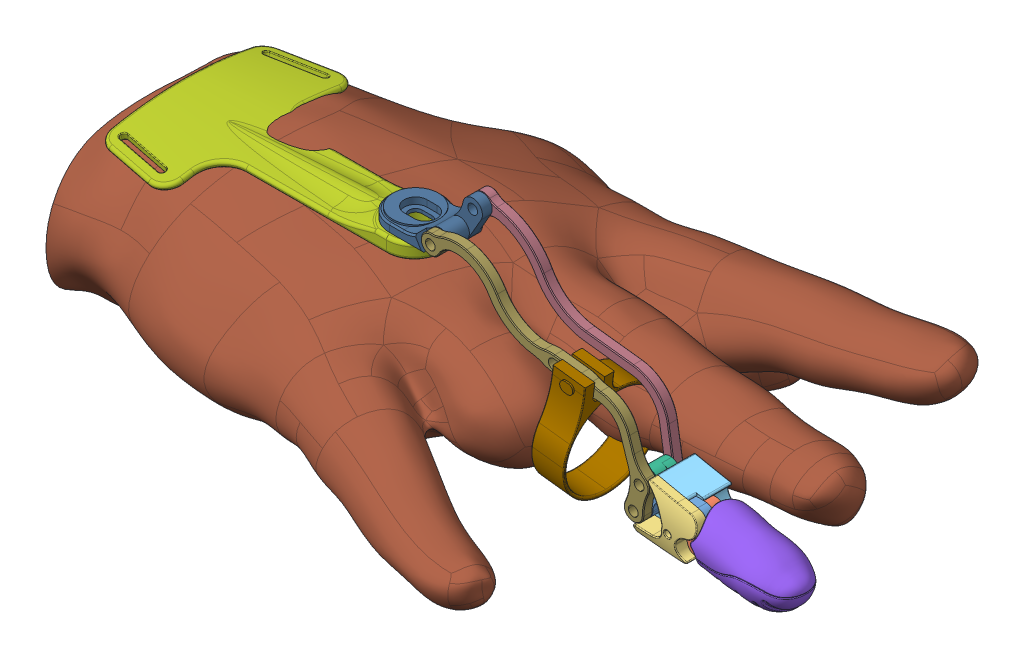
SolidWorks assembly Main assembly, configuration По умолчанию. Lengths in mm.
Overall size (204.71 145.18 159.08).
15 component instances, 13 part files, 0 mates.
Components (placement in the parent):
- Main assembly.STEP-1: Main assembly.STEP [По умолчанию] at origin size (204.71 145.18 159.08)
  - Mechanism_По умолчанию.STEP-1: Mechanism_По умолчанию.STEP [По умолчанию] at (125.6528 -29.2337 -1.5) x (0.984028 -0.178013 0) z (0 0 1) size (28.95 17.49 17.55)
    - Link_По умолчанию.STEP-1: Link_По умолчанию.STEP [По умолчанию] at (-0.3452 0.0075 0) x (0.999989 -0.004598 0) z (0 0 1) size (21.13 13.42 3)
    - Distal_По умолчанию.STEP-1: Distal_По умолчанию.STEP [По умолчанию] at (0.0408 -0.7405 0) x (0.998972 0.045334 0) z (0 0 1) size (13.04 12.89 6)
    - H-Fairing_По умолчанию.STEP-1: H-Fairing_По умолчанию.STEP [По умолчанию] at origin size (18.7 17.32 7.01)
    - Silicon pad_По умолчанию.STEP-1: Silicon pad_По умолчанию.STEP [По умолчанию] at origin size (15.4 12.02 9.54)
    - Fairing with silicon pad_По умолчанию.STEP-1: Fairing with silicon pad_По умолчанию.STEP [По умолчанию] at origin size (20.12 17.32 13.01)
    - Main_По умолчанию.STEP-1: Main_По умолчанию.STEP [По умолчанию] at origin size (23 13.47 9)
  - Wrist plate_По умолчанию.STEP-1: Wrist plate_По умолчанию.STEP [По умолчанию] at origin size (85.66 7.5 58.96)
  - Distal phalange_По умолчанию.STEP-1: Distal phalange_По умолчанию.STEP [По умолчанию] at (141.9491 -29.4551 4) x (-0.991086 0.133221 0) z (0 0 -1) size (28.35 16.07 17.47)
  - New Ring New_По умолчанию.STEP-1: New Ring New_По умолчанию.STEP [По умолчанию] at (101.1046 -20.5069 3.5) x (0 0 -1) z (0.992993 -0.118177 0) size (55.59 41.26 10)
  - Base new_v2_По умолчанию.STEP-1: Base new_v2_По умолчанию.STEP [По умолчанию] at (51 7.5 4) size (27 12.93 16)
  - Слепок руки_По умолчанию.STEP-1: Слепок руки_По умолчанию.STEP [По умолчанию] at (-28.867 -40.9581 -6.5474) x (-0.030677 0.930739 0.364394) z (0.998874 0.04175 -0.022547) size (97.22 128.09 195.46)
  - shatun 1 new_По умолчанию.STEP-1: shatun 1 new_По умолчанию.STEP [По умолчанию] at (50.1236 7.0074 8.5) x (0.999276 0.038056 0) z (0 0 1) size (68.82 49.18 3)
  - shatun 2 new_По умолчанию.STEP-1: shatun 2 new_По умолчанию.STEP [По умолчанию] at (125.6254 -29.2563 -0.5) x (-0.975639 0.219383 0) z (0 0 -1) size (72.79 38.16 3)
